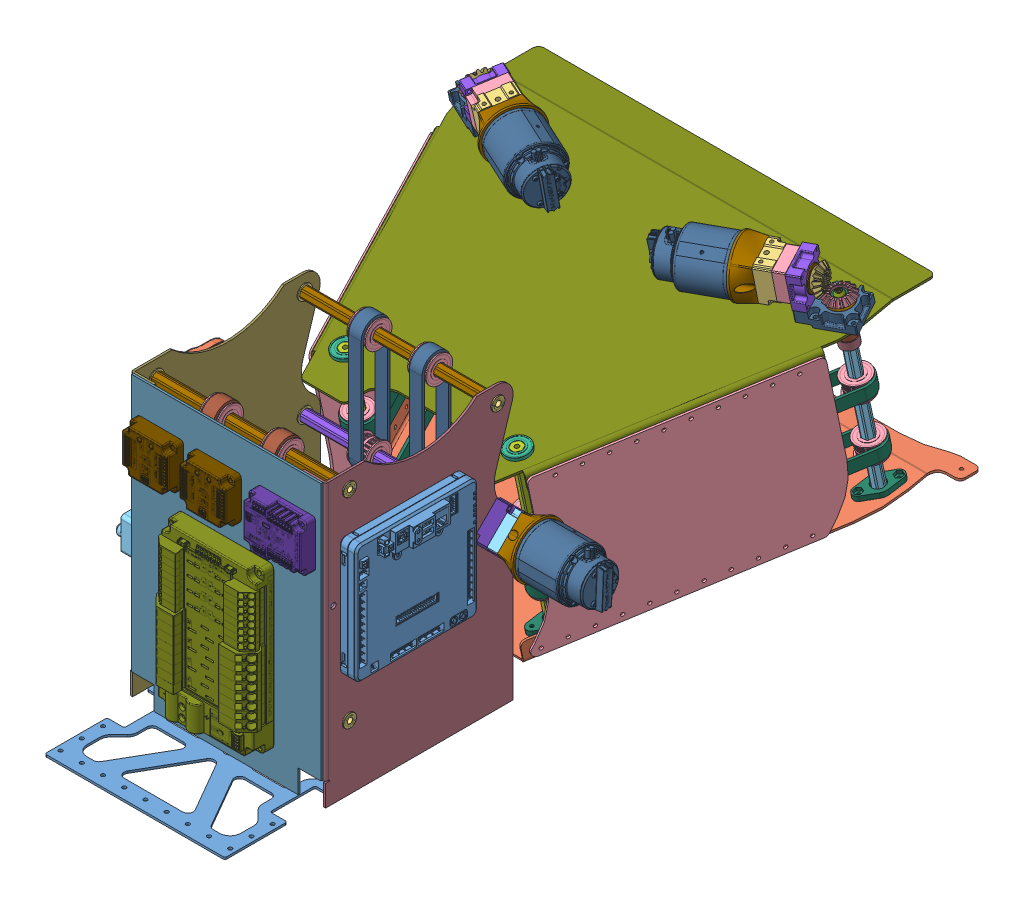
SolidWorks assembly 1250-20-FUNNELUPTAKE, configuration Default. Lengths in mm.
Overall size (535.62 401.79 765.58).
185 component instances, 60 part files, 56 mates.
Components (placement in the parent):
- CollectorBase-1: CollectorBase [Default] at (0 50.8 812.8) size (228.6 38.44 382.83)
- FunnelBottom-1: FunnelBottom [Default] at (0 55.0134 579.5904) x (-1 0 0) z (0 0 -1) size (530.22 177.8 749.3)
- Conveyor_Adjustable_Front-1: Conveyor_Adjustable_Front [Left] at (-217.1397 151.5504 137.6366) x (0.374607 -0.192772 0.906923) z (0 -0.978148 -0.207912) size (367.97 184.95 284.5)
  - 4262T370_PRECISION FLANGED BALL BEARING-1: 4262T370_PRECISION FLANGED BALL BEARING [4262T37] at (0 0 1.4732) x (0.649786 0.760118 0) z (0 0 1) size (17.53 17.53 4.98)
  - 217-4100-1: 217-4100 [Default] at (0 0 -52.5) size (32 32 22)
  - 217-4100-2: 217-4100 [Default] at (0 0 -125.3) x (0.973593 -0.228291 0) z (0 0 1) size (32 32 22)
  - 217-4100-3: 217-4100 [Default] at (304.9967 0 -52.5) x (-1 0 0) z (0 0 -1) size (32 32 22)
  - 217-4100-4: 217-4100 [Default] at (304.9967 0 -125.3) x (-1 0 0) z (0 0 -1) size (32 32 22)
  - 4262T370_PRECISION FLANGED BALL BEARING-2: 4262T370_PRECISION FLANGED BALL BEARING [4262T37] at (304.9967 0 1.4732) x (-0.209139 -0.977886 0) z (0 0 1) size (17.53 17.53 4.98)
  - 1250-20-D8006-1: 1250-20-D8006 [Default] at (0 0 -458.216) x (-0.999735 -0.023032 0) z (0 0 1) size (13.74 12.75 179.61)
  - Bearings-2: Bearings [217-4006] at (304.9967 0 -209.55) x (0.786149 -0.618036 0) z (0 0 1) size (31.12 31.12 7.95)
  - 1250-20-D8005-1: 1250-20-D8005 [Default] at (304.9967 0 -458.216) x (-0.964256 -0.264973 0) z (0 0 1) size (13.74 12.75 208.53)
  - 1250-20-D8004-1: 1250-20-D8004 [Default] at (20.8208 -20.8208 -244.04) x (-0.707107 -0.707107 0) z (0 0 -1) size (67.92 193.64 108.41)
    - 217-6293-000 Rev1-1: 217-6293-000 Rev1 [Default] at origin size (47.55 66.93 59.67)
      - 217-6293-001 Rev4-1: 217-6293-001 Rev4 [Default] at origin size (42 15.8 42)
      - 217-2742-001 Rev4_1-1: 217-2742-001 Rev4_1 [Default] at (0 1.5 0) x (0 1 0) z (-0.180103 0 0.983648) size (7 28 28)
      - 217-6293-002 Rev4-1: 217-6293-002 Rev4 [Default] at (0 21.7226 -21) x (-1 0 0) z (0 -1 0) size (42 17.3 57.45)
      - 217-2741-001 Rev4-1: 217-2741-001 Rev4 [Default] at (0 29.4451 -34.3) x (0 0 1) z (-1 0 0) size (5 26 26)
      - 217-6293-003 Rev2_217-3344 Rev7-1: 217-6293-003 Rev2_217-3344 Rev7 [Default] at (0 29.464 0) x (0.964719 0 -0.263283) z (0 1 0) size (34.55 34.81 34.49)
      - 217-6293-004 Rev1_217-3344 Rev7-1: 217-6293-004 Rev1_217-3344 Rev7 [Default] at (0 29.4451 -0.0551) x (0.856739 -0.515751 0) z (0 0 1) size (34.55 34.81 12.38)
      - 217-6293-005 Rev2-1: 217-6293-005 Rev2 [Default] at (0 29.4451 -25.1579) size (19 19 20.9)
      - 217-2742-001 Rev4_1-2: 217-2742-001 Rev4_1 [Default] at (0 29.4451 -28.0079) x (0 0 1) z (-0.091938 -0.995765 0) size (7 28 28)
      - 217-6293-006 Rev1-1: 217-6293-006 Rev1 [Default] at (0 29.4451 -13.3406) x (0.934686 0.355474 0) z (-0.355474 0.934686 0) size (15 1 15)
      - #.25-20 BHS, Grade 8 Steel Rev1_SBS2520-0375ZB-1: #.25-20 BHS, Grade 8 Steel Rev1_SBS2520-0375ZB [Default] at (0 29.4451 -22.8656) x (0.318453 -0.947939 0) z (0 0 1) size (11.17 11.19 13.79)
      - 217-2742-001 Rev4_1-3: 217-2742-001 Rev4_1 [Default] at (0 -6.7921 0) x (0 1 0) z (-0.180103 0 0.983648) size (7 28 28)
      - 217-2625-017 Rev1_9714K61_1-1: 217-2625-017 Rev1_9714K61_1 [Default] at (0.0233 0.2079 -0.2906) x (0.945176 0 0.326561) z (-0.326561 0 0.945176) size (28.51 4.98 30.18)
      - M4 SHCS, Grade 8 Steel_SSAM4-16MMZB-1: M4 SHCS, Grade 8 Steel_SSAM4-16MMZB [Default] at (12.7 3 -15.3) size (7 7 20.17)
      - M4 SHCS, Grade 8 Steel_SSAM4-16MMZB-2: M4 SHCS, Grade 8 Steel_SSAM4-16MMZB [Default] at (-12.7 -2 -15.3) x (0.984178 0.177185 0) z (0 0 1) size (7 7 20.17)
      - 217-2625-018 Rev1_98541A410_1-1: 217-2625-018 Rev1_98541A410_1 [Default] at (0 -7.3966 0) x (0 1 0) z (0 0 1) size (1 19.6 17.4)
      - 217-6293-007 Rev2_91595A074-1: 217-6293-007 Rev2_91595A074 [Default] at (-12.7 3.5 -20.1101) x (0 0 1) z (-1 0 0) size (16 3 3)
      - 217-6293-007 Rev2_91595A074-2: 217-6293-007 Rev2_91595A074 [Default] at (12.7 -2.5 -20.1101) x (0 0 1) z (-0.993885 -0.110422 0) size (16 3 3)
      - 217-2625-017 Rev1_9714K61_1-2: 217-2625-017 Rev1_9714K61_1 [Default] at (-0.0256 29.1668 -28.3002) x (0.987605 -0.156908 0.004131) z (-0.156909 -0.987613 -0.000027) size (28.51 4.98 30.18)
    - VersaPlanetary Input Blocks_VP Input Block-1: VersaPlanetary Input Blocks_VP Input Block [Default] at (-0.3528 -19.7 0.3459) x (0.019965 0 -0.999801) z (0 -1 0) size (44.45 42 18)
      - 217-2625-025 Rev1_1-1: 217-2625-025 Rev1_1 [Default] at (0 0 10.5) size (44.45 42 18)
    - VersaPlanetary Output Blocks_VP Output Block-1: VersaPlanetary Output Blocks_VP Output Block [Default] at (0 29.4451 -38.3) x (0 1 0) z (0 0 1)
    - VersaPlanetary Output Shafts_0.500 Hex (217-2615-003)-1: VersaPlanetary Output Shafts_0.500 Hex (217-2615-003) [Default] at (0 29.4451 -38.3875) x (-0.745957 -0.665994 0) z (0 0 -1)
    - VersaPlanetary Ring Gears_VP Ring Gear-1: VersaPlanetary Ring Gears_VP Ring Gear [Default] at (0 -7 0) x (0 0 -1) z (0 1 0)
    - 217-2816-001 Rev1_1-1: 217-2816-001 Rev1_1 [Default] at (-0.3528 -13.35 0.3459) x (0.019965 0 -0.999801) z (0 1 0) size (42 42 14.5)
    - VersaPlanetary Gear Sets_10_1 (217-2820)-1: VersaPlanetary Gear Sets_10_1 (217-2820) [Default] at (-2.3011 -54.2671 25.511) x (0.966683 0 0.255977) z (0 1 0) size (48.18 46.59 17.81)
      - 217-2820-000 Rev2_Public-1: 217-2820-000 Rev2_Public [Default] at (-4.3058 25.2501 42.9205) x (-0.964009 -0.265871 0) z (0 0 -1) size (39.26 38.9 17.81)
        - 217-2625-100_1-1: 217-2625-100_1 [Default] at origin size (39.26 38.9 12.7)
          - 217-2625-008 Rev1-1: 217-2625-008 Rev1 [Default] at origin size (34.7 34.7 4.7)
          - 217-2625-010 Rev1-1: 217-2625-010 Rev1 [Default] at (0 10.193 3.65) x (0.999813 0.019336 0) z (0 0 1) size (4 4 12)
          - 217-2625-010 Rev1-2: 217-2625-010 Rev1 [Default] at (8.691 -5.3258 3.65) size (4 4 12)
          - 217-2625-010 Rev1-3: 217-2625-010 Rev1 [Default] at (-8.691 -5.3258 3.65) size (4 4 12)
          - 217-2625-005 Rev1_Planet_Revolving_Follower01-1: 217-2625-005 Rev1_Planet_Revolving_Follower01 [Default] at (8.691 -5.3258 6.35) x (0.932816 0.360354 0) z (0 0 1) size (16.91 16.92 8)
          - 217-2625-005 Rev1_Planet_Revolving_Follower01-2: 217-2625-005 Rev1_Planet_Revolving_Follower01 [Default] at (-8.691 -5.3258 6.35) x (-0.932788 -0.360426 0) z (0 0 1) size (16.91 16.92 8)
          - 217-2625-005 Rev1_Planet_Revolving_Follower01-3: 217-2625-005 Rev1_Planet_Revolving_Follower01 [Default] at (0 10.193 6.35) x (0.893583 0.448898 0) z (0 0 1) size (16.91 16.92 8)
        - 217-2625-007 Rev6_Sun_Driver01-1: 217-2625-007 Rev6_Sun_Driver01 [Default] at (0 0 6.7) size (14.49 14.49 13.12)
    - 217-4018-1: 217-4018 [Default] at (-0.3528 -47.525 0.3459) x (0.999801 0 0.019965) z (-0.019965 0 0.999801) size (64 21.67 64)
    - Motors-1: Motors [217-6515] at (-0.3528 -59.05 0.3459) x (0 -1 0) z (0.020556 0 0.999789) size (116.05 66.49 70.16)
    - 217-5839-1-1: 217-5839-1 [Default] at (0 29.4451 -43.6603) x (-0.997272 -0.073818 0) z (0 0 -1) size (22.58 22.1 42.62)
      - 217-5839-001 Rev6-1: 217-5839-001 Rev6 [Default] at origin size (18 18 32.62)
      - 217-5839-005 Rev1_91251A148-1: 217-5839-005 Rev1_91251A148 [Default] at (0 0 1.5524) x (-0.465417 -0.885092 0) z (0 0 -1) size (5.74 5.74 16.4)
      - 217-5839-006 Rev4-1: 217-5839-006 Rev4 [Default] at (0 0 18.2524) x (0.993768 0.111469 0) z (0 0 1) size (20 20 18)
      - 217-4649-007 Rev1_94105A824-1: 217-4649-007 Rev1_94105A824 [Default] at (9.1095 1.0218 24.0024) x (0.016297 -0.145289 -0.989255) z (0.993768 0.111469 0) size (4.83 4.83 4.9)
  - Belt1-10-1: Belt1-10 [Default] at (304.9967 0 -52.5) size (339.65 34.65 15)
  - Belt1-10-2: Belt1-10 [Default] at (304.9967 0 -125.3) size (339.65 34.65 15)
- Conveyor_Adjustable_Front-3: Conveyor_Adjustable_Front [Default] at (217.1397 151.5504 137.6366) x (-0.374607 -0.192772 0.906923) z (0 -0.978148 -0.207912) size (367.52 184.95 284.5)
  - 4262T370_PRECISION FLANGED BALL BEARING-1: 4262T370_PRECISION FLANGED BALL BEARING [4262T37] at (0 0 1.4732) x (0.649786 0.760118 0) z (0 0 1) size (17.53 17.53 4.98)
  - 217-4100-1: 217-4100 [Default] at (0 0 -52.5) size (32 32 22)
  - 217-4100-2: 217-4100 [Default] at (0 0 -125.3) x (0.973593 -0.228291 0) z (0 0 1) size (32 32 22)
  - 217-4100-3: 217-4100 [Default] at (304.9967 0 -52.5) x (-1 0 0) z (0 0 -1) size (32 32 22)
  - 217-4100-4: 217-4100 [Default] at (304.9967 0 -125.3) x (-1 0 0) z (0 0 -1) size (32 32 22)
  - 4262T370_PRECISION FLANGED BALL BEARING-2: 4262T370_PRECISION FLANGED BALL BEARING [4262T37] at (304.9967 0 1.4732) x (-0.209139 -0.977886 0) z (0 0 1) size (17.53 17.53 4.98)
  - 1250-20-D8006-1: 1250-20-D8006 [Default] at (0 0 -458.216) x (-0.999735 -0.023032 0) z (0 0 1) size (13.74 12.75 179.61)
  - Bearings-2: Bearings [217-4006] at (304.9967 0 -209.55) x (0.786149 -0.618036 0) z (0 0 1) size (31.12 31.12 7.95)
  - 1250-20-D8005-1: 1250-20-D8005 [Default] at (304.9967 0 -458.216) x (-0.964256 -0.264973 0) z (0 0 1) size (13.74 12.75 208.53)
  - 1250-20-D8004-1: 1250-20-D8004 [Default] at (20.8208 20.8208 -244.04) x (0.707107 -0.707107 0) z (0 0 -1) size (67.92 193.64 108.41)
    - 217-6293-000 Rev1-1: 217-6293-000 Rev1 [Default] at origin size (47.55 66.93 59.67)
      - 217-6293-001 Rev4-1: 217-6293-001 Rev4 [Default] at origin size (42 15.8 42)
      - 217-2742-001 Rev4_1-1: 217-2742-001 Rev4_1 [Default] at (0 1.5 0) x (0 1 0) z (-0.180103 0 0.983648) size (7 28 28)
      - 217-6293-002 Rev4-1: 217-6293-002 Rev4 [Default] at (0 21.7226 -21) x (-1 0 0) z (0 -1 0) size (42 17.3 57.45)
      - 217-2741-001 Rev4-1: 217-2741-001 Rev4 [Default] at (0 29.4451 -34.3) x (0 0 1) z (-1 0 0) size (5 26 26)
      - 217-6293-003 Rev2_217-3344 Rev7-1: 217-6293-003 Rev2_217-3344 Rev7 [Default] at (0 29.464 0) x (0.964719 0 -0.263283) z (0 1 0) size (34.55 34.81 34.49)
      - 217-6293-004 Rev1_217-3344 Rev7-1: 217-6293-004 Rev1_217-3344 Rev7 [Default] at (0 29.4451 -0.0551) x (0.856739 -0.515751 0) z (0 0 1) size (34.55 34.81 12.38)
      - 217-6293-005 Rev2-1: 217-6293-005 Rev2 [Default] at (0 29.4451 -25.1579) size (19 19 20.9)
      - 217-2742-001 Rev4_1-2: 217-2742-001 Rev4_1 [Default] at (0 29.4451 -28.0079) x (0 0 1) z (-0.091938 -0.995765 0) size (7 28 28)
      - 217-6293-006 Rev1-1: 217-6293-006 Rev1 [Default] at (0 29.4451 -13.3406) x (0.934686 0.355474 0) z (-0.355474 0.934686 0) size (15 1 15)
      - #.25-20 BHS, Grade 8 Steel Rev1_SBS2520-0375ZB-1: #.25-20 BHS, Grade 8 Steel Rev1_SBS2520-0375ZB [Default] at (0 29.4451 -22.8656) x (0.318453 -0.947939 0) z (0 0 1) size (11.17 11.19 13.79)
      - 217-2742-001 Rev4_1-3: 217-2742-001 Rev4_1 [Default] at (0 -6.7921 0) x (0 1 0) z (-0.180103 0 0.983648) size (7 28 28)
      - 217-2625-017 Rev1_9714K61_1-1: 217-2625-017 Rev1_9714K61_1 [Default] at (0.0233 0.2079 -0.2906) x (0.945176 0 0.326561) z (-0.326561 0 0.945176) size (28.51 4.98 30.18)
      - M4 SHCS, Grade 8 Steel_SSAM4-16MMZB-1: M4 SHCS, Grade 8 Steel_SSAM4-16MMZB [Default] at (12.7 3 -15.3) size (7 7 20.17)
      - M4 SHCS, Grade 8 Steel_SSAM4-16MMZB-2: M4 SHCS, Grade 8 Steel_SSAM4-16MMZB [Default] at (-12.7 -2 -15.3) x (0.984178 0.177185 0) z (0 0 1) size (7 7 20.17)
      - 217-2625-018 Rev1_98541A410_1-1: 217-2625-018 Rev1_98541A410_1 [Default] at (0 -7.3966 0) x (0 1 0) z (0 0 1) size (1 19.6 17.4)
      - 217-6293-007 Rev2_91595A074-1: 217-6293-007 Rev2_91595A074 [Default] at (-12.7 3.5 -20.1101) x (0 0 1) z (-1 0 0) size (16 3 3)
      - 217-6293-007 Rev2_91595A074-2: 217-6293-007 Rev2_91595A074 [Default] at (12.7 -2.5 -20.1101) x (0 0 1) z (-0.993885 -0.110422 0) size (16 3 3)
      - 217-2625-017 Rev1_9714K61_1-2: 217-2625-017 Rev1_9714K61_1 [Default] at (-0.0256 29.1668 -28.3002) x (0.987605 -0.156908 0.004131) z (-0.156909 -0.987613 -0.000027) size (28.51 4.98 30.18)
    - VersaPlanetary Input Blocks_VP Input Block-1: VersaPlanetary Input Blocks_VP Input Block [Default] at (-0.3528 -19.7 0.3459) x (0.019965 0 -0.999801) z (0 -1 0) size (44.45 42 18)
      - 217-2625-025 Rev1_1-1: 217-2625-025 Rev1_1 [Default] at (0 0 10.5) size (44.45 42 18)
    - VersaPlanetary Output Blocks_VP Output Block-1: VersaPlanetary Output Blocks_VP Output Block [Default] at (0 29.4451 -38.3) x (0 1 0) z (0 0 1)
    - VersaPlanetary Output Shafts_0.500 Hex (217-2615-003)-1: VersaPlanetary Output Shafts_0.500 Hex (217-2615-003) [Default] at (0 29.4451 -38.3875) x (-0.745957 -0.665994 0) z (0 0 -1)
    - VersaPlanetary Ring Gears_VP Ring Gear-1: VersaPlanetary Ring Gears_VP Ring Gear [Default] at (0 -7 0) x (0 0 -1) z (0 1 0)
    - 217-2816-001 Rev1_1-1: 217-2816-001 Rev1_1 [Default] at (-0.3528 -13.35 0.3459) x (0.019965 0 -0.999801) z (0 1 0) size (42 42 14.5)
    - VersaPlanetary Gear Sets_10_1 (217-2820)-1: VersaPlanetary Gear Sets_10_1 (217-2820) [Default] at (-2.3011 -54.2671 25.511) x (0.966683 0 0.255977) z (0 1 0) size (48.18 46.59 17.81)
      - 217-2820-000 Rev2_Public-1: 217-2820-000 Rev2_Public [Default] at (-4.3058 25.2501 42.9205) x (-0.964009 -0.265871 0) z (0 0 -1) size (39.26 38.9 17.81)
        - 217-2625-100_1-1: 217-2625-100_1 [Default] at origin size (39.26 38.9 12.7)
          - 217-2625-008 Rev1-1: 217-2625-008 Rev1 [Default] at origin size (34.7 34.7 4.7)
          - 217-2625-010 Rev1-1: 217-2625-010 Rev1 [Default] at (0 10.193 3.65) x (0.999813 0.019336 0) z (0 0 1) size (4 4 12)
          - 217-2625-010 Rev1-2: 217-2625-010 Rev1 [Default] at (8.691 -5.3258 3.65) size (4 4 12)
          - 217-2625-010 Rev1-3: 217-2625-010 Rev1 [Default] at (-8.691 -5.3258 3.65) size (4 4 12)
          - 217-2625-005 Rev1_Planet_Revolving_Follower01-1: 217-2625-005 Rev1_Planet_Revolving_Follower01 [Default] at (8.691 -5.3258 6.35) x (0.932816 0.360354 0) z (0 0 1) size (16.91 16.92 8)
          - 217-2625-005 Rev1_Planet_Revolving_Follower01-2: 217-2625-005 Rev1_Planet_Revolving_Follower01 [Default] at (-8.691 -5.3258 6.35) x (-0.932788 -0.360426 0) z (0 0 1) size (16.91 16.92 8)
          - 217-2625-005 Rev1_Planet_Revolving_Follower01-3: 217-2625-005 Rev1_Planet_Revolving_Follower01 [Default] at (0 10.193 6.35) x (0.893583 0.448898 0) z (0 0 1) size (16.91 16.92 8)
        - 217-2625-007 Rev6_Sun_Driver01-1: 217-2625-007 Rev6_Sun_Driver01 [Default] at (0 0 6.7) size (14.49 14.49 13.12)
    - 217-4018-1: 217-4018 [Default] at (-0.3528 -47.525 0.3459) x (0.999801 0 0.019965) z (-0.019965 0 0.999801) size (64 21.67 64)
    - Motors-1: Motors [217-6515] at (-0.3528 -59.05 0.3459) x (0 -1 0) z (0.020556 0 0.999789) size (116.05 66.49 70.16)
    - 217-5839-1-1: 217-5839-1 [Default] at (0 29.4451 -43.6603) x (-0.997272 -0.073818 0) z (0 0 -1) size (22.58 22.1 42.62)
      - 217-5839-001 Rev6-1: 217-5839-001 Rev6 [Default] at origin size (18 18 32.62)
      - 217-5839-005 Rev1_91251A148-1: 217-5839-005 Rev1_91251A148 [Default] at (0 0 1.5524) x (-0.465417 -0.885092 0) z (0 0 -1) size (5.74 5.74 16.4)
      - 217-5839-006 Rev4-1: 217-5839-006 Rev4 [Default] at (0 0 18.2524) x (0.993768 0.111469 0) z (0 0 1) size (20 20 18)
      - 217-4649-007 Rev1_94105A824-1: 217-4649-007 Rev1_94105A824 [Default] at (9.1095 1.0218 24.0024) x (0.016297 -0.145289 -0.989255) z (0.993768 0.111469 0) size (4.83 4.83 4.9)
  - Belt1-10-1: Belt1-10 [Default] at (304.9967 0 -52.5) size (339.65 34.65 15)
  - Belt1-10-2: Belt1-10 [Default] at (304.9967 0 -125.3) size (339.65 34.65 15)
- FunnelTop-1: FunnelTop [Default] at (0 255.2527 627.0933) x (1 0 0) z (0 0.406737 -0.913545) size (476.25 100.05 408.43)
- Conveyor_Adjustable-4: Conveyor_Adjustable [Default] at (0 240.8033 495.3) x (0 1 0) z (-1 0 0) size (215.46 136.52 367.03)
  - 4262T370_PRECISION FLANGED BALL BEARING-1: 4262T370_PRECISION FLANGED BALL BEARING [4262T37] at (0 0 115.7732) x (0.362925 0.931819 0) z (0 0 1) size (17.53 17.53 4.98)
  - 217-4100-1: 217-4100 [Default] at (0 0 36.4) x (0 -1 0) z (0 0 1) size (32 32 22)
  - 217-4100-2: 217-4100 [Default] at (0 0 -36.4) x (0.935356 -0.353707 0) z (0 0 1) size (32 32 22)
  - 217-4100-3: 217-4100 [Default] at (127.4967 0 36.4) x (0 -1 0) z (0 0 -1) size (32 32 22)
  - 217-4100-4: 217-4100 [Default] at (127.4967 0 -36.4) x (-0.30191 0.953336 0) z (0 0 -1) size (32 32 22)
  - 4262T370_PRECISION FLANGED BALL BEARING-2: 4262T370_PRECISION FLANGED BALL BEARING [4262T37] at (127.4967 0 115.7732) x (0.547561 -0.836766 0) z (0 0 1) size (17.53 17.53 4.98)
  - 1250-20-D8005-1: 1250-20-D8005 [Default] at (-15.7154 -15.7154 -133.465) x (0 0 1) z (-0.707107 0.707107 0) size (151 96.65 96.43)
    - 217-2625-026 Rev1-1: 217-2625-026 Rev1 [Default] at (-6.5 22.225 0) x (0 -1 0) z (-1 0 0) size (44.45 42 18.13)
    - 217-2742-001 Rev4-1: 217-2742-001 Rev4 [Default] at (0.2002 22.225 0) x (1 0 0) z (0 -0.092627 0.995701) size (7 28 28)
    - 217-2742-001 Rev4-2: 217-2742-001 Rev4 [Default] at (8.2002 22.225 0) size (7 28 28)
    - 217-2625-017 Rev1_9714K61-1: 217-2625-017 Rev1_9714K61 [Default] at (7.42 22.3002 -0.342) x (0 0.56703 0.823697) z (0 -0.823697 0.56703) size (28.51 4.98 30.18)
    - 217-2625-018 Rev1_98541A410-1: 217-2625-018 Rev1_98541A410 [Default] at (-0.7046 22.225 0) x (1 0 0) z (0 -0.017452 0.999848) size (1 19.6 17.4)
    - 832-1750-Ring-Gear-Screw_SSA0832-0500ZC-1: 832-1750-Ring-Gear-Screw_SSA0832-0500ZC [Default] at (-30.7 4.725 -17.5) x (0 0.997447 0.071411) z (0 -0.071411 0.997447) size (6.73 48.51 6.73)
    - 832-1750-Ring-Gear-Screw_SSA0832-0500ZC-2: 832-1750-Ring-Gear-Screw_SSA0832-0500ZC [Default] at (-30.7 39.725 17.5) x (0 0.005929 0.999982) z (0 -0.999982 0.005929) size (6.73 48.51 6.73)
    - 217-2820 Rev1_Public-1: 217-2820 Rev1_Public [Default] at (-4.6546 22.225 0) x (0 -0.456494 0.889726) z (-1 0 0) size (39.26 38.9 17.4)
      - 217-2625-100-1: 217-2625-100 [Default] at origin size (39.26 38.9 12.7)
        - 217-2625-008 Rev1-1: 217-2625-008 Rev1 [Default] at origin size (34.7 34.7 4.7)
        - 217-2625-010 Rev1-1: 217-2625-010 Rev1 [Default] at (0 10.193 3.65) x (0.999813 0.019336 0) z (0 0 1) size (4 4 12)
        - 217-2625-010 Rev1-2: 217-2625-010 Rev1 [Default] at (8.691 -5.3258 3.65) size (4 4 12)
        - 217-2625-010 Rev1-3: 217-2625-010 Rev1 [Default] at (-8.691 -5.3258 3.65) size (4 4 12)
        - 217-2625-005 Rev1_Planet_Revolving_Follower01-1: 217-2625-005 Rev1_Planet_Revolving_Follower01 [Default] at (8.691 -5.3258 6.35) x (0.932816 0.360354 0) z (0 0 1) size (16.91 16.92 8)
        - 217-2625-005 Rev1_Planet_Revolving_Follower01-2: 217-2625-005 Rev1_Planet_Revolving_Follower01 [Default] at (-8.691 -5.3258 6.35) x (-0.932788 -0.360426 0) z (0 0 1) size (16.91 16.92 8)
        - 217-2625-005 Rev1_Planet_Revolving_Follower01-3: 217-2625-005 Rev1_Planet_Revolving_Follower01 [Default] at (0 10.193 6.35) x (0.893583 0.448898 0) z (0 0 1) size (16.91 16.92 8)
      - 217-2625-007 Rev1_Public-1: 217-2625-007 Rev1_Public [Default] at (0 0 6.7) x (0.992772 0.120019 0) z (0 0 1) size (14.49 14.49 12.72)
    - 217-2816-001 Rev1-1: 217-2816-001 Rev1 [Default] at (-6.35 22.225 0) x (0 -1 0) z (1 0 0) size (42 42 14.5)
    - 217-4649-001 Rev1-1: 217-4649-001 Rev1 [Default] at (-20.046 22.225 0) x (0 -1 0) z (1 0 0) size (18 18 13)
    - 217-4649-007 Rev1_94105A824-1: 217-4649-007 Rev1_94105A824 [Default] at (-25.521 22.225 -6.7835) x (-0.996104 -0.088191 0) z (0 0 -1) size (4.83 4.83 4.9)
    - 217-2625-011 Rev1-1: 217-2625-011 Rev1 [Default] at (-24.7818 22.225 0) x (0 0 1) z (0 -1 0) size (8.01 7.5 7.94)
    - 217-4018-1: 217-4018 [Default] at (-22.525 22.225 0) x (0 0 1) z (0 1 0) size (64 21.67 64)
    - 217-5839-001 Rev6-1: 217-5839-001 Rev6 [Default] at (7.4478 22.225 0) x (0 0.929438 -0.368979) z (1 0 0) size (18 18 32.62)
    - 217-5839-006 Rev4-1: 217-5839-006 Rev4 [Default] at (25.7002 22.225 0) x (0 0.707107 -0.707107) z (1 0 0) size (20 20 18)
    - Motors-1: Motors [217-6515] at (-34.05 22.225 0) x (-1 0 0) z (0 0.736791 -0.67612) size (116.05 66.49 70.16)
  - 1250-20-D8007-1: 1250-20-D8007 [Default] at (0 0 -343.916) x (0.999747 0.022501 0) z (0 0 1) size (13.74 12.75 219.55)
  - 1250-20-D8008-1: 1250-20-D8008 [Default] at (127.4967 0 -343.916) x (0.251755 0.967791 0) z (0 0 1) size (13.74 12.75 226.57)
  - 4262T370_PRECISION FLANGED BALL BEARING-3: 4262T370_PRECISION FLANGED BALL BEARING [4262T37] at (127.4967 0 -115.7732) x (0.380122 -0.924936 0) z (0 0 -1) size (17.53 17.53 4.98)
  - Belt-2-1: Belt-2 [Default] at (0 0 36.4) size (162.15 34.65 15)
  - Belt-2-2: Belt-2 [Default] at (0 0 -36.4) size (162.15 34.65 15)
- Conveyor_Adjustable_WallBack-1: Conveyor_Adjustable_WallBack [Default] at (0 116.3007 673.1) x (0 1 0) z (-1 0 0) size (282.08 44.13 236.52)
  - 4262T370_PRECISION FLANGED BALL BEARING-1: 4262T370_PRECISION FLANGED BALL BEARING [4262T37] at (12.0026 0 115.7732) x (-0.994896 0.100906 0) z (0 0 1) size (17.53 17.53 4.98)
  - 217-4100-1: 217-4100 [Default] at (12.0026 0 36.4) size (32 32 22)
  - 217-4100-2: 217-4100 [Default] at (12.0026 0 -36.4) x (0.846245 0.532793 0) z (0 0 1) size (32 32 22)
  - 217-4100-3: 217-4100 [Default] at (251.9993 0 36.4) x (0 -1 0) z (0 0 -1) size (32 32 22)
  - 217-4100-4: 217-4100 [Default] at (251.9993 0 -36.4) x (-0.955152 -0.296114 0) z (0 0 -1) size (32 32 22)
  - 4262T370_PRECISION FLANGED BALL BEARING-2: 4262T370_PRECISION FLANGED BALL BEARING [4262T37] at (251.9993 0 115.7732) x (-0.685256 0.728302 0) z (0 0 1) size (17.53 17.53 4.98)
  - 1250-20-D8008-1: 1250-20-D8008 [Default] at (12.0026 0 -343.916) x (0.892369 0.451307 0) z (0 0 1) size (13.74 12.75 226.57)
  - 1250-20-D8008-2: 1250-20-D8008 [Default] at (251.9993 0 -343.916) size (13.74 12.75 226.57)
  - 4262T370_PRECISION FLANGED BALL BEARING-3: 4262T370_PRECISION FLANGED BALL BEARING [4262T37] at (12.0026 0 -115.7732) x (0.956772 -0.29084 0) z (0 0 -1) size (17.53 17.53 4.98)
  - 4262T370_PRECISION FLANGED BALL BEARING-4: 4262T370_PRECISION FLANGED BALL BEARING [4262T37] at (251.9993 0 -115.7732) x (-0.317925 0.948116 0) z (0 0 -1) size (17.53 17.53 4.98)
  - Belt-3-1: Belt-3 [Default] at (12.0026 0 36.4) size (274.65 34.65 15)
  - Belt-3-2: Belt-3 [Default] at (12.0026 0 -36.4) size (274.65 34.65 15)
- SidePanelLeft-1: SidePanelLeft [Default] at (-114.3 50.8 586.74) x (0 0 -1) z (0 -1 0) size (224.79 27.94 336.55)
- SidePanel-1: SidePanel [Left] at (116.84 50.8 586.74) x (0 0 -1) z (0 -1 0) size (224.79 27.94 336.55)
- SidePanelRight-1: SidePanelRight [Default] at (0.0254 211.1375 701.04) x (1 0 0) z (0 -1 0) size (227.08 2.54 336.55)
- pinkball (^_^.)-1: pinkball (^_^.) [Default] at (26.3103 216.4279 259.9973) x (0.970476 0.239396 0.029438) z (0.146002 -0.680201 0.718338) size (177.8 177.8 177.8) (hidden)
- bearingholder-1: bearingholder [Default] at (-217.1397 151.5504 137.6366) x (0.374607 -0.192772 0.906923) z (-0.927184 -0.077885 0.366421) size (50.8 6.35 25.4)
- bearingholder-2: bearingholder [Default] at (-102.8859 92.7554 414.245) x (0.374607 -0.192772 0.906923) z (-0.927184 -0.077885 0.366421) size (50.8 6.35 25.4)
- bearingholder-3: bearingholder [Default] at (102.8859 98.9667 415.5652) x (-0.374607 -0.192772 0.906923) z (0.927184 -0.077885 0.366421) size (50.8 6.35 25.4)
- bearingholder-4: bearingholder [Default] at (217.1397 151.5504 137.6366) x (-0.374607 -0.192772 0.906923) z (-0.927184 0.077885 -0.366421) size (50.8 6.35 25.4)
- Electrical-1: Electrical [Default] at (0 0.0011 0) size (293.58 266.83 244.43)
  - 217-4244-1: 217-4244 [Default] at (0.0254 183.2046 710.2602) x (0 1 0) z (1 0 0) size (192.68 36.15 120.93)
  - 217-4243-1: 217-4243 [Default] at (72.6695 320.802 708.025) x (1 0 0) z (0 -1 0) size (69.09 19.67 56.9)
  - 217-4245-1: 217-4245 [Default] at (-9.349 325.3848 710.686) x (1 0 0) z (0 -1 0) size (56.39 19.92 51.56)
  - 217-4245-2: 217-4245 [Default] at (-78.437 325.3848 710.686) x (1 0 0) z (0 -1 0) size (56.39 19.92 51.56)
  - AM-3000-1: AM-3000 [Default] at (126.492 252.3051 612.2147) x (0 0 -1) z (1 0 0) size (146.27 143.19 34.5)
  - RobotRadio-1: RobotRadio [Default] at (-116.84 279.5026 659.766) x (0 1 0) z (0 0 1) size (69.89 25.47 95.8)
  - Part1-1: Part1 [Default] at (-116.84 149.3049 419.3534) x (0 -1 0) z (-1 0 0) size (120.65 88.9 25.4)
- 1250-20-D8010-2: 1250-20-D8010 [Default] at (-182.4466 309.3664 345.6171) x (0.927184 0.077885 -0.366421) z (-0.374607 0.192772 -0.906923) size (2.54 198.12 306.84)
- 1250-20-D8010-1: 1250-20-D8010 [Default] at (182.4466 309.3664 345.6171) x (0.927184 -0.077885 0.366421) z (0.374607 0.192772 -0.906923) size (2.54 198.12 306.84)
- MainCircuitBreaker_120A-1: MainCircuitBreaker_120A [Default] at (-121.92 196.2666 660.9334) x (0 0 1) z (-1 0 0) size (50.95 73.41 44.2)
Mates (geometry in assembly coordinates):
- Symmetric1: symmetric: plane of CollectorBase-1 through (107.95 48.26 812.8) normal (1 0 0); plane of CollectorBase-1 through (-107.95 48.26 812.8) normal (-1 0 0); plane of assembly
- Coincident1: coincident: plane of CollectorBase-1 through (-107.95 48.26 812.8) normal (0 0 1); plane of assembly through (0 0 812.8) normal (0 0 1)
- Distance1: distance = 50.8 mm: plane of assembly through (0 0 0) normal (0 1 0); plane of CollectorBase-1 through (0 50.8 812.8) normal (0 1 0)
- Coincident6: coincident: point of FunnelBottom-1; plane of assembly
- Coincident7: coincident: plane of FunnelBottom-1 through (-254 159.1534 101.867) normal (0 0.978148 0.207912); plane of Conveyor_Adjustable_Front-1/4262T370_PRECISION FLANGED BALL BEARING-1 through (-222.4942 152.1293 134.913) normal (0 -0.978148 -0.207912)
- Coincident8: coincident: plane of CollectorBase-1 through (0 6.3792 808.3966) normal (0 0.978148 0.207912); plane of FunnelBottom-1 through (-254 156.6689 101.3389) normal (0 -0.978148 -0.207912)
- Symmetric5: symmetric: plane of Conveyor_Adjustable-4/217-4100-1 through (-25.775 240.8033 495.3) normal (1 0 0); plane of Conveyor_Adjustable-4/217-4100-2 through (25.775 240.8033 495.3) normal (-1 0 0)
- Coincident22: coincident: plane of CollectorBase-1 through (0 50.8 812.8) normal (0 1 0); plane of SidePanelLeft-1 through (-116.84 50.8 476.25) normal (0 -1 0)
- Coincident39: coincident: plane of SidePanelLeft-1 through (-116.84 387.35 495.3) normal (0 1 0); plane of SidePanelRight-1 through (113.5634 387.35 703.58) normal (0 1 0)
- Coincident40: coincident: plane of SidePanelLeft-1 through (-114.3 50.8 701.04) normal (0 0 1); plane of SidePanelRight-1 through (0.0254 211.1375 701.04) normal (0 0 -1)
- Tangent10: tangent: plane of FunnelBottom-1 through (-254 159.1534 101.867) normal (0 0.978148 0.207912); sphere of pinkball (^_^.)-1
- Coincident61: coincident: plane of FunnelBottom-1 through (-254 159.1534 101.867) normal (0 0.978148 0.207912); plane of bearingholder-1 through (-217.1397 151.5504 137.6366) normal (0 -0.978148 -0.207912)
- Coincident62: coincident: plane of FunnelBottom-1 through (-254 159.1534 101.867) normal (0 0.978148 0.207912); plane of bearingholder-2 through (-102.8859 92.7554 414.245) normal (0 -0.978148 -0.207912)
- Symmetric6: symmetric: plane of Conveyor_Adjustable_WallBack-1 through (0 116.3007 673.1) normal (0 0 -1); plane of Conveyor_Adjustable-4 through (0 240.8033 495.3) normal (0 0 -1); plane of assembly
- Distance20: distance = 88.9 mm: plane of Conveyor_Adjustable-4 through (0 240.8033 495.3) normal (0 0 -1); plane of assembly through (0 0 584.2) normal (0 0 1)
- Distance21: distance = 25.4 mm: line of FunnelBottom-1 through (-111.125 82.8979 460.6209) axis (-0.374607 0.192772 -0.906923); plane of Conveyor_Adjustable_Front-1 through (-217.1397 151.5504 137.6366) normal (-0.927184 -0.077885 0.366421)
- Coincident69: coincident: plane of FunnelBottom-1 through (0 55.0134 579.5904) normal (-1 0 0); plane of assembly through (0 0 0) normal (1 0 0)
- Coincident70: coincident: plane of FunnelBottom-1 through (-254 159.1534 101.867) normal (0 0.978148 0.207912); plane of Conveyor_Adjustable_Front-3/4262T370_PRECISION FLANGED BALL BEARING-1 through (215.2221 152.7402 132.0391) normal (0 -0.978148 -0.207912)
- Coincident73: coincident: plane of FunnelBottom-1 through (0 149.0659 137.1085) normal (0 -0.207912 0.978148); point of Conveyor_Adjustable_Front-3
- Coincident74: coincident: plane of FunnelBottom-1 through (0 149.0659 137.1085) normal (0 -0.207912 0.978148); point of Conveyor_Adjustable_Front-1
- Concentric31: concentric: cylinder of FunnelBottom-1 through (-217.1397 70.9792 120.5106) axis (0 0.978148 0.207912) radius 7.9375; cylinder of bearingholder-1 through (-217.1397 157.7616 138.9568) axis (0 -0.978148 -0.207912) radius 7.9375
- Concentric32: concentric: cylinder of FunnelBottom-1 through (-102.8859 12.1843 397.119) axis (0 0.978148 0.207912) radius 7.9375; cylinder of bearingholder-2 through (-102.8859 98.9667 415.5652) axis (0 -0.978148 -0.207912) radius 7.9375
- Distance24: distance = 317.5 mm: plane of Conveyor_Adjustable-4/217-4100-3 through (-36.4 368.3 495.3) normal (0 -1 0); plane of CollectorBase-1 through (0 50.8 812.8) normal (0 1 0)
- Coincident76: coincident: plane of Conveyor_Adjustable-4/217-4100-3 through (-36.4 368.3 495.3) normal (0 -1 0); plane of Conveyor_Adjustable_WallBack-1/217-4100-3 through (-36.4 368.3 673.1) normal (0 -1 0)
- Distance25: distance = 203.2 mm: plane of FunnelTop-1 through (-31.75 284.298 490.4461) normal (0 -0.978148 -0.207912); plane of FunnelBottom-1 through (-254 159.1534 101.867) normal (0 0.978148 0.207912)
- Coincident78: coincident: plane of FunnelTop-1 through (0 255.2527 627.0933) normal (1 0 0); plane of assembly through (0 0 0) normal (1 0 0)
- Distance27: distance = 25.4 mm: plane of Conveyor_Adjustable_WallBack-1 through (0 116.3007 673.1) normal (0 0 -1); plane of SidePanelLeft-1 through (-114.3 50.8 698.5) normal (0 0 -1)
- Parallel16: parallel: plane of FunnelBottom-1 through (-254 75.8652 97.5978) normal (-0.927184 -0.077885 0.366421); plane of bearingholder-1 through (-217.1397 151.5504 137.6366) normal (-0.927184 -0.077885 0.366421)
- Parallel17: parallel: plane of bearingholder-1 through (-217.1397 151.5504 137.6366) normal (-0.927184 -0.077885 0.366421); plane of bearingholder-2 through (-102.8859 92.7554 414.245) normal (-0.927184 -0.077885 0.366421)
- Concentric33: concentric: cylinder of FunnelBottom-1 through (217.1397 68.3964 119.9617) axis (0 0.978148 0.207912) radius 7.9375; cylinder of Conveyor_Adjustable_Front-3/4262T370_PRECISION FLANGED BALL BEARING-1 through (217.1397 147.6746 136.8127) axis (0 -0.978148 -0.207912) radius 7.9375
- Coincident831: coincident: plane of FunnelBottom-1 through (-254 159.1534 101.867) normal (0 0.978148 0.207912); plane of bearingholder-3 through (102.8859 92.7554 414.245) normal (0 -0.978148 -0.207912)
- Coincident841: coincident: plane of FunnelBottom-1 through (-254 159.1534 101.867) normal (0 0.978148 0.207912); plane of bearingholder-4 through (217.1397 151.5504 137.6366) normal (0 -0.978148 -0.207912)
- Concentric34: concentric: cylinder of Conveyor_Adjustable_Front-3/4262T370_PRECISION FLANGED BALL BEARING-1 through (217.1397 152.5442 137.8478) axis (0 0.978148 0.207912) radius 8.763; cylinder of bearingholder-4 through (217.1397 157.7616 138.9568) axis (0 -0.978148 -0.207912) radius 7.9375
- Parallel20: parallel: plane of bearingholder-3 through (102.8859 98.9667 415.5652) normal (0.927184 -0.077885 0.366421); plane of bearingholder-4 through (217.1397 151.5504 137.6366) normal (-0.927184 0.077885 -0.366421)
- Coincident842: coincident: plane of Conveyor_Adjustable_WallBack-1 through (0 116.3007 673.1) normal (-1 0 0); plane of assembly through (0 0 0) normal (1 0 0)
- Symmetric7: symmetric: plane of SidePanelLeft-1 through (-116.84 240.8033 495.3) normal (-1 0 0); plane of SidePanel-1 through (116.84 240.8033 495.3) normal (1 0 0); plane of assembly
- Coincident843: coincident: plane of SidePanelLeft-1 through (-114.3 50.8 586.74) normal (0 -1 0); plane of SidePanel-1 through (116.84 50.8 586.74) normal (0 -1 0)
- Coincident844: coincident: plane of SidePanelLeft-1 through (-114.3 50.8 586.74) normal (0 0 -1); plane of SidePanel-1 through (116.84 50.8 586.74) normal (0 0 -1)
- Coincident845: coincident: plane of FunnelBottom-1 through (-254 82.8979 460.6209) normal (0 -0.207912 0.978148); plane of FunnelTop-1 through (-111.125 284.142 503.3967) normal (0 -0.207912 0.978148)
- Coincident846: coincident: plane of Electrical-1 through (0 0.0011 0) normal (1 0 0); plane of assembly through (0 0 0) normal (1 0 0)
- Coincident847: coincident: plane of SidePanelRight-1 through (0.0254 211.1375 703.58) normal (0 0 1); plane of Electrical-1/217-4244-1 through (57.4294 275.2299 703.58) normal (0 0 -1)
- Concentric36: concentric: cylinder of FunnelBottom-1 through (217.1397 68.3964 119.9617) axis (0 0.978148 0.207912) radius 7.9375; cylinder of Conveyor_Adjustable_Front-3/4262T370_PRECISION FLANGED BALL BEARING-1 through (217.1397 147.6746 136.8127) axis (0 -0.978148 -0.207912) radius 7.9375
- Concentric37: concentric: cylinder of FunnelBottom-1 through (224.2759 152.7382 119.8316) axis (0 0.978148 0.207912) radius 2.0955; cylinder of bearingholder-4 through (224.2759 161.4339 121.6799) axis (0 -0.978148 -0.207912) radius 2.0955
- Concentric38: concentric: cylinder of FunnelBottom-1 through (102.8859 9.6015 396.5701) axis (0 0.978148 0.207912) radius 7.9375; cylinder of Conveyor_Adjustable_Front-3/4262T370_PRECISION FLANGED BALL BEARING-2 through (102.8859 88.8796 413.4211) axis (0 -0.978148 -0.207912) radius 7.9375
- Concentric39: concentric: cylinder of FunnelBottom-1 through (110.0222 93.9433 396.44) axis (0 0.978148 0.207912) radius 2.0955; cylinder of bearingholder-3 through (110.0222 96.4278 396.9681) axis (0 0.978148 0.207912) radius 2.0955
- Concentric40: concentric: cylinder of FunnelBottom-1 through (95.7497 86.5986 430.9938) axis (0 0.978148 0.207912) radius 2.0955; cylinder of bearingholder-3 through (95.7497 89.0831 431.5219) axis (0 0.978148 0.207912) radius 2.0955
- Coincident848: coincident: plane of FunnelTop-1 through (-56.1301 250.5377 649.2758) normal (-0.927184 -0.077885 0.366421); plane of 1250-20-D8010-2 through (-181.2691 309.4653 345.1517) normal (0.927184 0.077885 -0.366421)
- Coincident849: coincident: plane of FunnelTop-1 through (-233.3201 319.3591 215.5459) normal (-0.374607 0.192772 -0.906923); plane of 1250-20-D8010-2 through (-233.3201 339.2351 219.7707) normal (-0.374607 0.192772 -0.906923)
- Coincident850: coincident: line of FunnelTop-1 through (-233.3201 339.2351 219.7707) axis (0.374607 -0.192772 0.906923); plane of 1250-20-D8010-2 through (-233.3201 339.2351 219.7707) normal (0 0.978148 0.207912)
- Coincident852: coincident: plane of FunnelBottom-1 through (57.8087 50.1574 602.4362) normal (0.927184 -0.077885 0.366421); plane of 1250-20-D8010-1 through (181.2691 309.4653 345.1517) normal (-0.927184 0.077885 -0.366421)
- Coincident853: coincident: plane of 1250-20-D8010-1 through (235.6751 339.0373 220.7014) normal (0.374607 0.192772 -0.906923); plane of FunnelTop-1 through (233.3201 341.7196 220.2988) normal (0.374607 0.192772 -0.906923)
- Coincident854: coincident: line of FunnelTop-1 through (128.655 285.3745 473.1649) axis (0.374607 0.192772 -0.906923); plane of 1250-20-D8010-1 through (235.6751 339.0373 220.7014) normal (0 0.978148 0.207912)
- Distance29: distance = 31.75 mm: line of Electrical-1/217-4244-1 through (-52.1679 82.55 703.8384) axis (1 0 0); plane of CollectorBase-1 through (0 50.8 812.8) normal (0 1 0)
- Coincident858: coincident: plane of SidePanelLeft-1 through (-116.84 240.8033 495.3) normal (-1 0 0); plane of MainCircuitBreaker_120A-1 through (-116.84 232.9696 685.0634) normal (1 0 0)
- Distance30: distance = 12.7 mm: plane of MainCircuitBreaker_120A-1 through (-121.92 232.9696 685.0634) normal (0 0 1); line of SidePanelLeft-1 through (-116.84 78.6765 697.7634) axis (0 1 0)
- Coincident860: coincident: plane of CollectorBase-1 through (-114.3 48.26 684.2125) normal (-1 0 0); plane of SidePanelLeft-1 through (-114.3 240.8033 495.3) normal (1 0 0)
